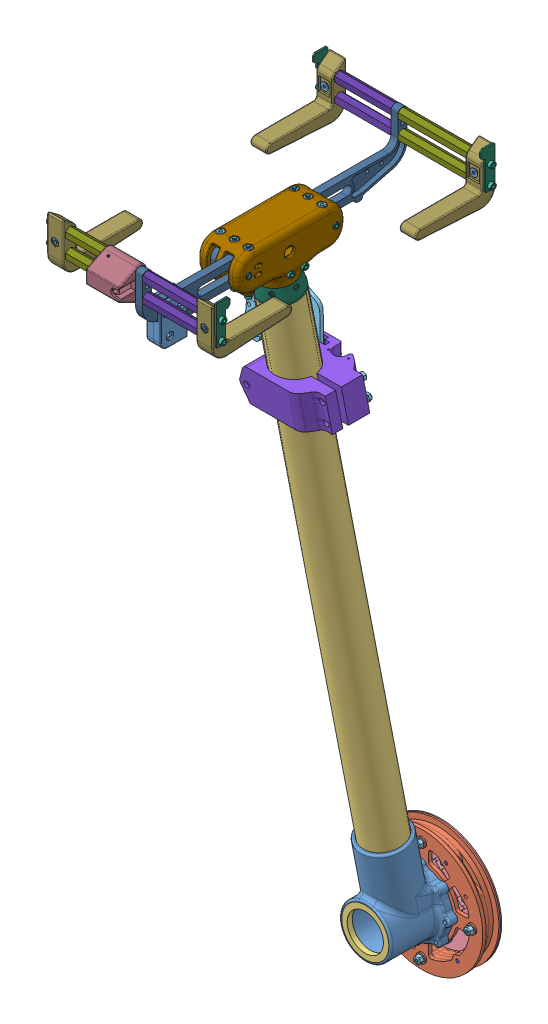
SolidWorks assembly 971-18-A-4600_Distal Arm Tubes, configuration Default. Lengths in mm.
Overall size (268.43 1098.92 452.33).
183 component instances, 51 part files, 58 mates.
Components (placement in the parent):
- 971-18-P-0131_Distal Joint End Sleeve Block-1: 971-18-P-0131_Distal Joint End Sleeve Block [Default] at origin size (98.43 160.77 84.48)
- 971-18-P-0117_Distal Joint Capstan Top -1: 971-18-P-0117_Distal Joint Capstan Top  [Distal Joint Capstan Top] at (47.625 -11.95 -3.3338) x (0 0 1) z (-0.707107 0.707107 0) size (24.51 167.64 167.64)
- 50mm x 65mm x 7mm-1: 50mm x 65mm x 7mm [Default] at (47.625 -11.95 5.3975) x (0 0 1) z (-0.033242 -0.999447 0) size (7 65 65)
- 971-18-A-2800_Capstan Tensioner-1: 971-18-A-2800_Capstan Tensioner [Default] at (81.152 21.577 -3.3338) x (0.707107 -0.707107 0) z (0 0 -1) size (57.15 30.16 17.27)
  - 971-18-P-0066_Capstan Tensioner Block-1: 971-18-P-0066_Capstan Tensioner Block [Default] at origin size (57.15 9.53 17.27)
  - Nylon-Insert Locknut-1: Nylon-Insert Locknut [#10-32  Nylon-Insert Locknut] at (-20.6375 2.032 0) x (-0.5 0 -0.866025) z (-0.866025 0 0.5) size (9.53 5.95 11)
  - SHCS-2: SHCS [0.875, #10-32] at (-20.6375 -1.5875 0) x (0 -1 0) z (-0.804306 0 -0.594216) size (27.05 7.92 7.92)
  - Nylon-Insert Locknut-2: Nylon-Insert Locknut [#10-32  Nylon-Insert Locknut] at (20.6375 2.032 0) x (0.5 0 -0.866025) z (-0.866025 0 -0.5) size (9.53 5.95 11)
  - SHCS-3: SHCS [0.875, #10-32] at (20.6375 -1.5875 0) x (0 -1 0) z (-0.804306 0 0.594216) size (27.05 7.92 7.92)
  - 3-16 in wire rope stop-1: 3-16 in wire rope stop [Default] at (5.4991 13.4938 0) x (0.991815 0 0.127683) z (-0.127683 0 0.991815) size (10.72 7.94 10.72)
  - 3-16 in wire rope stop-2: 3-16 in wire rope stop [Default] at (-5.4991 13.4938 0) x (0.997136 0 0.075631) z (-0.075631 0 0.997136) size (10.72 7.94 10.72)
- 50mm x 65mm x 7mm-2: 50mm x 65mm x 7mm [Default] at (47.625 -11.95 81.4369) x (0 0 1) z (-0.807978 0.589212 0) size (7 65 65)
- Dowel Pins-1: Dowel Pins [0.1875" OD, 0.5" Length] at (17.3166 -42.2584 11.7475) x (0 0 1) z (0.811004 0.585041 0) size (12.7 4.76 4.76)
- SHCS-1: SHCS [0.375, #10-32] at (4.7625 -11.95 10.16) x (0 0 1) z (0.375926 0.92665 0) size (14.35 7.92 7.92)
- Dowel Pins-8: Dowel Pins [0.1875" OD, 0.5" Length] at (77.9334 -42.2584 11.7475) x (0 0 1) z (-0.585041 0.811004 0) size (12.7 4.76 4.76)
- Dowel Pins-9: Dowel Pins [0.1875" OD, 0.5" Length] at (77.9334 18.3584 11.7475) x (0 0 1) z (-0.811004 -0.585041 0) size (12.7 4.76 4.76)
- Dowel Pins-10: Dowel Pins [0.1875" OD, 0.5" Length] at (17.3166 18.3584 11.7475) x (0 0 1) z (0.585041 -0.811004 0) size (12.7 4.76 4.76)
- SHCS-8: SHCS [0.375, #10-32] at (47.625 -54.8125 10.16) x (0 0 1) z (-0.92665 0.375926 0) size (14.35 7.92 7.92)
- SHCS-9: SHCS [0.375, #10-32] at (90.4875 -11.95 10.16) x (0 0 1) z (-0.375926 -0.92665 0) size (14.35 7.92 7.92)
- SHCS-10: SHCS [0.375, #10-32] at (47.625 30.9125 10.16) x (0 0 1) z (0.92665 -0.375926 0) size (14.35 7.92 7.92)
- 971-18-A-4000_The Claw-1: 971-18-A-4000_The Claw [Default] at (47.625 881.6358 218.1087) x (-1 0 0) z (0 -0.000724 1) size (243.27 530.53 410.02)
  - 971-18-P-0108_Printed Claw Body-1: 971-18-P-0108_Printed Claw Body [Default] at origin size (58.05 92.05 149.22)
  - 971-18-P-0077_Main Claw plate-2: 971-18-P-0077_Main Claw plate [Main Claw plate revised] at (9.4298 -158.75 -26.9875) x (0 0 1) z (-1 0 0) size (261.94 82.88 9.53)
  - 971-18-P-0077_Main Claw plate-3: 971-18-P-0077_Main Claw plate [Main Claw plate revised] at (-9.4298 -158.75 26.9875) x (0 0 -1) z (1 0 0) size (261.94 82.88 9.53)
  - SHCS-1: SHCS [2.25, #10-32] at (3.175 0 -60.325) x (1 0 0) z (0 0.140282 0.990112) size (61.98 7.92 7.92)
  - SHCS-2: SHCS [2.25, #10-32] at (3.175 0 60.325) x (1 0 0) z (0 0.980553 -0.196257) size (61.98 7.92 7.92)
  - SHCS-3: SHCS [1.875, #10-32] at (-19.177 -1.5875 -50.8) x (0 -1 0) z (-0.074372 0 -0.997231) size (52.45 7.92 7.92)
  - SHCS-8: SHCS [2.25, #10-32] at (0 1.5875 -50.8) x (0 -1 0) z (-0.997477 0 -0.07099) size (61.98 7.92 7.92)
  - SHCS-9: SHCS [2.25, #10-32] at (19.177 1.5875 -50.8) x (0 -1 0) z (-0.818231 0 -0.57489) size (61.98 7.92 7.92)
  - SHCS-10: SHCS [1.875, #10-32] at (19.177 -1.5875 50.8) x (0 -1 0) z (-0.72422 0 -0.689569) size (52.45 7.92 7.92)
  - SHCS-11: SHCS [2.25, #10-32] at (0 1.5875 50.8) x (0 -1 0) z (-0.999175 0 0.040609) size (61.98 7.92 7.92)
  - SHCS-12: SHCS [2.25, #10-32] at (-19.177 1.5875 50.8) x (0 -1 0) z (0.998979 0 0.045167) size (61.98 7.92 7.92)
  - 9433K640_PRECISION STAINLESS STEEL EXTENSION SPRING-1: 9433K640_PRECISION STAINLESS STEEL EXTENSION SPRING [9433K64] at (18.9548 0 -18.9695) x (0 0 1) z (-1 0 0) size (39.67 9.89 9.66)
  - 91259A155_ALLOY STEEL SHOULDER SCREW-1: 91259A155_ALLOY STEEL SHOULDER SCREW [91259A155] at (20.5423 0 -7.9375) x (0 -0.354679 -0.934988) z (0 -0.934988 0.354679) size (6.35 13.86 6.35)
  - 91259A155_ALLOY STEEL SHOULDER SCREW-2: 91259A155_ALLOY STEEL SHOULDER SCREW [91259A155] at (-20.5423 0 -34.9538) x (0 -0.751431 0.659812) z (0 -0.659812 -0.751431) size (6.35 13.86 6.35)
  - 9433K640_PRECISION STAINLESS STEEL EXTENSION SPRING-2: 9433K640_PRECISION STAINLESS STEEL EXTENSION SPRING [9433K64] at (-18.9548 0 20.6375) x (0 0 1) z (-1 0 0) size (39.67 9.89 9.66)
  - Bearings-1: Bearings [0.1875 ID, 0.375 OD, 0.125 Width, R166-2Z] at (9.3662 27.94 -18.3873) x (0 -0.996654 0.08174) z (1 0 0) size (9.53 9.53 3.17)
  - Bearings-2: Bearings [0.1875 ID, 0.375 OD, 0.125 Width, R166-2Z] at (-9.4932 27.94 1.0215) x (0 -0.380852 0.924636) z (1 0 0) size (9.53 9.53 3.17)
  - 971-18-P-0120_Printed Claw Pulley-3: 971-18-P-0120_Printed Claw Pulley [Default] at (-9.4298 27.94 1.0215) x (0 0.87562 0.483001) z (-1 0 0) size (19.05 19.05 4.76)
  - 971-18-P-0120_Printed Claw Pulley-4: 971-18-P-0120_Printed Claw Pulley [Default] at (9.4298 27.94 -18.3873) x (0 -0.06152 0.998106) z (-1 0 0) size (19.05 19.05 4.76)
  - SHCS-13: SHCS [2.25, #10-32] at (3.175 27.94 -18.3873) x (1 0 0) z (0 0.140282 0.990112) size (61.98 7.92 7.92)
  - SHCS-14: SHCS [2.25, #10-32] at (3.175 27.94 1.0215) x (1 0 0) z (0 0.140282 0.990112) size (61.98 7.92 7.92)
  - Nylon-Insert Locknut-1: Nylon-Insert Locknut [#10-32 Thin Nylon-Insert Locknut] at (22.225 27.94 1.0215) x (0 -0.5 -0.866025) z (0 -0.866025 0.5) size (9.53 4.37 11)
  - Nylon-Insert Locknut-2: Nylon-Insert Locknut [#10-32 Thin Nylon-Insert Locknut] at (22.225 27.94 -18.3873) x (0 1 0) z (0 0 -1) size (9.53 4.37 11)
  - Nylon-Insert Locknut-4: Nylon-Insert Locknut [#10-32 Thin Nylon-Insert Locknut] at (24.2094 0 -60.325) x (0 -0.5 -0.866025) z (0 -0.866025 0.5) size (9.53 4.37 11)
  - Nylon-Insert Locknut-5: Nylon-Insert Locknut [#10-32 Thin Nylon-Insert Locknut] at (24.2094 0 60.325) x (0 -0.5 0.866025) z (0 0.866025 0.5) size (9.53 4.37 11)
  - Nylon-Insert Locknut-14: Nylon-Insert Locknut [#10-32 Thin Nylon-Insert Locknut] at (19.177 -21.0344 50.8) x (0.5 0 0.866025) z (0.866025 0 -0.5) size (9.53 4.37 11)
  - Nylon-Insert Locknut-15: Nylon-Insert Locknut [#10-32 Thin Nylon-Insert Locknut] at (0 -21.0344 50.8) x (-0.5 0 -0.866025) z (-0.866025 0 0.5) size (9.53 4.37 11)
  - Nylon-Insert Locknut-17: Nylon-Insert Locknut [#10-32 Thin Nylon-Insert Locknut] at (-19.177 -21.0344 50.8) x (-0.5 0 -0.866025) z (-0.866025 0 0.5) size (9.53 4.37 11)
  - Nylon-Insert Locknut-18: Nylon-Insert Locknut [#10-32 Thin Nylon-Insert Locknut] at (0 -21.0344 -50.8) x (1 0 0) z (0 0 -1) size (9.53 4.37 11)
  - Nylon-Insert Locknut-19: Nylon-Insert Locknut [#10-32 Thin Nylon-Insert Locknut] at (-19.177 -21.0344 -50.8) x (0.5 0 -0.866025) z (-0.866025 0 -0.5) size (9.53 4.37 11)
  - Nylon-Insert Locknut-20: Nylon-Insert Locknut [#10-32 Thin Nylon-Insert Locknut] at (19.177 -21.0344 -50.8) x (-0.5 0 0.866025) z (0.866025 0 0.5) size (9.53 4.37 11)
  - 971-18-P-0142_Distal Carbon tube adapter-1: 971-18-P-0142_Distal Carbon tube adapter [Default] at (0 89.7497 -17.5007) x (-0.5 -0.165748 -0.850016) z (0 0.981514 -0.19139) size (53.98 53.98 46.99)
  - 6498K084_ROUND BODY AIR CYLINDER-1: 6498K084_ROUND BODY AIR CYLINDER [6498K084] at (0 262.1497 -57.0582) x (0 0.981514 -0.19139) z (0 0.19139 0.981514) size (365.16 28.45 28.45)
  - 5779K652_PUSH-TO-CONNECT TUBE FITTING FOR AIR-1: 5779K652_PUSH-TO-CONNECT TUBE FITTING FOR AIR [5779K652] at (0 225.7462 -44.6778) x (-1 0 0) z (0 -0.19139 -0.981514) size (14.22 28.59 25.52)
  - 971-18-P-0153_Claw Piston Mount-1: 971-18-P-0153_Claw Piston Mount [Default] at (0 207.2186 -46.3469) x (-1 0 0) z (0 -0.19139 -0.981514) size (45.75 3.17 41.53)
  - FHCS-15: FHCS [0.25, #4-40] at (-15.7499 209.7238 -50.0883) x (-0.913608 0.077818 0.39908) z (0 0.981514 -0.19139) size (6.48 6.48 6.43)
  - FHCS-18: FHCS [0.25, #4-40] at (15.7499 209.7238 -50.0883) x (-0.453098 0.170616 0.874981) z (0 0.981514 -0.19139) size (6.48 6.48 6.43)
  - FHCS-17: FHCS [0.25, #4-40] at (0 214.9449 -23.313) x (-0.453098 0.170616 0.874981) z (0 0.981514 -0.19139) size (6.48 6.48 6.43)
  - 971-18-P-0162_Claw Piston Cable Block-1: 971-18-P-0162_Claw Piston Cable Block [Default] at (0 80.0327 -21.5464) x (0.973108 0.044086 0.22609) z (-0.230348 0.186243 0.95512) size (12.7 31.75 12.7)
  - SHCS-19: SHCS [0.875, #10-32] at (0.7167 71.3508 -22.9383) x (0.230348 -0.186243 -0.95512) z (0.455328 -0.84681 0.274935) size (27.05 7.92 7.92)
  - Nylon-Insert Locknut-21: Nylon-Insert Locknut [#10-32 Thin Nylon-Insert Locknut] at (1.843 70.4402 -27.6084) x (-0.550845 -0.834076 0.029792) z (0.802191 -0.51926 0.294719) size (9.53 4.37 11)
  - SAE Washer, 18-8 Stainless Steel-1: SAE Washer, 18-8 Stainless Steel [No. 10 Screw SAE Washer] at (-1.6529 73.2667 -13.113) x (0.166548 0.974577 -0.14987) z (0.95875 -0.124551 0.25551) size (12.7 1.65 12.7)
  - SAE Washer, 18-8 Stainless Steel-2: SAE Washer, 18-8 Stainless Steel [No. 10 Screw SAE Washer] at (1.6529 70.5939 -26.8199) x (0.166548 0.974577 -0.14987) z (0.95875 -0.124551 0.25551) size (12.7 1.65 12.7)
  - FHCS-19: FHCS [0.25, #4-40] at (0 214.9449 -23.313) x (-0.309292 0.182005 0.933388) z (0 0.981514 -0.19139) size (6.48 6.48 6.43)
  - Beam Diffuse Sensor-1: Beam Diffuse Sensor [Default] at (2.3678 -35.946 191.135) x (0 -1 0) z (0 0 1) size (12.7 33.5 22.88)
  - SHCS-24: SHCS [1, #10-32] at (-103.6637 -29.5056 185.7375) x (1 0 0) z (0 0.235318 -0.971918) size (30.45 7.92 7.92)
  - SHCS-26: SHCS [1.5, #4-40] at (30.5617 -43.439 194.183) x (0 -1 0) z (0.977714 0 0.209939) size (40.94 4.65 4.65)
  - SHCS-33: SHCS [1, #10-32] at (103.6637 -29.5056 185.7375) x (-1 0 0) z (0 0.845438 -0.534073) size (30.45 7.92 7.92)
  - SHCS-35: SHCS [1, #10-32] at (103.6637 -54.9056 185.7375) x (-1 0 0) z (0 -0.631694 -0.775218) size (30.45 7.92 7.92)
  - SHCS-37: SHCS [1, #10-32] at (103.6637 -29.5056 -185.7375) x (-1 0 0) z (0 -0.058563 -0.998284) size (30.45 7.92 7.92)
  - SHCS-39: SHCS [1, #10-32] at (103.6637 -54.9056 -185.7375) x (-1 0 0) z (0 -0.744643 -0.667463) size (30.45 7.92 7.92)
  - SHCS-41: SHCS [1, #10-32] at (-103.6637 -54.9056 -185.7375) x (1 0 0) z (0 0.359883 -0.932997) size (30.45 7.92 7.92)
  - SHCS-43: SHCS [1, #10-32] at (-103.6637 -29.5056 -185.7375) x (1 0 0) z (0 0.980192 0.198051) size (30.45 7.92 7.92)
  - 92311A433_18-8 SS CUP POINT SET SCREW-1: 92311A433_18-8 SS CUP POINT SET SCREW [92311A433] at (-10.0105 -54.9056 185.7375) x (0 -0.712759 -0.701409) z (-1 0 0) size (4.99 4.84 25.82)
  - 92311A433_18-8 SS CUP POINT SET SCREW-5: 92311A433_18-8 SS CUP POINT SET SCREW [92311A433] at (-11.02 -29.5056 185.7375) x (0 -0.999929 0.011906) z (1 0 0) size (4.99 4.84 25.82)
  - 93365A142_BRASS HEAT-SET INSERT FOR PLASTICS-1: 93365A142_BRASS HEAT-SET INSERT FOR PLASTICS [93365A142] at (-11.1125 53.5447 9.169) x (0.785545 0.5 0.36458) z (0.36458 -0.850016 0.380203) size (6.35 8.46 6.35)
  - 93365A142_BRASS HEAT-SET INSERT FOR PLASTICS-2: 93365A142_BRASS HEAT-SET INSERT FOR PLASTICS [93365A142] at (-22.225 49.8609 -9.7226) x (0 0.545272 0.838259) z (0 -0.838259 0.545272) size (6.35 8.46 6.35)
  - 93365A142_BRASS HEAT-SET INSERT FOR PLASTICS-4: 93365A142_BRASS HEAT-SET INSERT FOR PLASTICS [93365A142] at (-11.1125 46.1772 -28.6142) x (-0.813186 -0.24774 0.526644) z (0.297873 -0.954543 0.010914) size (6.35 8.46 6.35)
  - 93365A142_BRASS HEAT-SET INSERT FOR PLASTICS-6: 93365A142_BRASS HEAT-SET INSERT FOR PLASTICS [93365A142] at (11.1125 46.1772 -28.6142) x (0.371763 0.927557 0.037811) z (-0.782172 0.33491 -0.525398) size (6.35 8.46 6.35)
  - 93365A142_BRASS HEAT-SET INSERT FOR PLASTICS-8: 93365A142_BRASS HEAT-SET INSERT FOR PLASTICS [93365A142] at (22.225 49.8609 -9.7226) x (0 0.873561 -0.486714) z (0 -0.486714 -0.873561) size (6.35 8.46 6.35)
  - 93365A142_BRASS HEAT-SET INSERT FOR PLASTICS-10: 93365A142_BRASS HEAT-SET INSERT FOR PLASTICS [93365A142] at (11.1125 53.5447 9.169) x (0.459987 0.780789 -0.422825) z (0.733766 -0.602409 -0.314152) size (6.35 8.46 6.35)
  - 92311A433_18-8 SS CUP POINT SET SCREW-11: 92311A433_18-8 SS CUP POINT SET SCREW [92311A433] at (9.2914 -29.5056 -185.7375) x (0 0.990314 -0.138846) z (1 0 0) size (4.99 4.84 25.82)
  - 92311A433_18-8 SS CUP POINT SET SCREW-14: 92311A433_18-8 SS CUP POINT SET SCREW [92311A433] at (9.9158 -54.9056 -185.7375) x (0 -0.994426 -0.105437) z (1 0 0) size (4.99 4.84 25.82)
  - 94638A222_NYLON UNTHREADED SPACERS-1: 94638A222_NYLON UNTHREADED SPACERS [94638A222] at (-19.177 0 50.8) x (1 0 0) z (0 1 0) size (9.53 9.53 33.34)
  - 94638A222_NYLON UNTHREADED SPACERS-2: 94638A222_NYLON UNTHREADED SPACERS [94638A222] at (-19.177 0 -50.8) x (1 0 0) z (0 1 0) size (9.53 9.53 33.34)
  - 94638A222_NYLON UNTHREADED SPACERS-3: 94638A222_NYLON UNTHREADED SPACERS [94638A222] at (19.177 0 -50.8) x (1 0 0) z (0 1 0) size (9.53 9.53 33.34)
  - 94639A550_NYLON UNTHREADED SPACERS-1: 94639A550_NYLON UNTHREADED SPACERS [94639A550] at (-9.4298 0 -60.325) x (0 -0.918334 -0.395806) z (1 0 0) size (12.7 12.7 9.53)
  - 94639A586_NYLON UNTHREADED SPACERS-1: 94639A586_NYLON UNTHREADED SPACERS [94639A586] at (0 11.9062 50.8) x (1 0 0) z (0 1 0) size (9.53 9.53 10.32)
  - 94638A222_NYLON UNTHREADED SPACERS-4: 94638A222_NYLON UNTHREADED SPACERS [94638A222] at (19.177 0 50.8) x (1 0 0) z (0 1 0) size (9.53 9.53 33.34)
  - 94639A550_NYLON UNTHREADED SPACERS-2: 94639A550_NYLON UNTHREADED SPACERS [94639A550] at (9.4298 0 -60.325) x (0 -0.323653 0.946176) z (-1 0 0) size (12.7 12.7 9.53)
  - 94639A550_NYLON UNTHREADED SPACERS-3: 94639A550_NYLON UNTHREADED SPACERS [94639A550] at (-9.4298 0 60.325) x (0 -0.362888 0.931833) z (-1 0 0) size (12.7 12.7 9.53)
  - 94639A550_NYLON UNTHREADED SPACERS-4: 94639A550_NYLON UNTHREADED SPACERS [94639A550] at (9.4298 0 60.325) x (0 -0.966697 0.255924) z (-1 0 0) size (12.7 12.7 9.53)
  - 94639A586_NYLON UNTHREADED SPACERS-2: 94639A586_NYLON UNTHREADED SPACERS [94639A586] at (0 11.9062 -50.8) x (1 0 0) z (0 1 0) size (9.53 9.53 10.32)
  - 94639A586_NYLON UNTHREADED SPACERS-3: 94639A586_NYLON UNTHREADED SPACERS [94639A586] at (0 -11.9062 50.8) x (1 0 0) z (0 1 0) size (9.53 9.53 10.32)
  - 94639A586_NYLON UNTHREADED SPACERS-4: 94639A586_NYLON UNTHREADED SPACERS [94639A586] at (0 -11.9062 -50.8) x (1 0 0) z (0 1 0) size (9.53 9.53 10.32)
  - 91780A049_ALUM FEM THRDED HEX STANDOFF-1: 91780A049_ALUM FEM THRDED HEX STANDOFF [91780A049] at (0 174.4329 -15.4133) x (0.203683 0.187378 0.960938) z (0 -0.981514 0.19139) size (6.35 7.33 76.64)
  - 98637A123_ALLOY STEEL MIL SPEC CUP POINT SET SCREW-1: 98637A123_ALLOY STEEL MIL SPEC CUP POINT SET SCREW [98637A123] at (0 134.5273 -7.632) x (0.994254 0.020488 0.105072) z (0 -0.981514 0.19139) size (3.28 2.93 13.1)
  - SHCS-44: SHCS [1, #10-32] at (-103.6637 -54.9056 185.7375) x (1 0 0) z (0 0.985655 0.168775) size (30.45 7.92 7.92)
  - 91780A049_ALUM FEM THRDED HEX STANDOFF-2: 91780A049_ALUM FEM THRDED HEX STANDOFF [91780A049] at (15.7499 94.4205 -27.6048) x (-0.911227 0.078834 0.404291) z (0 0.981514 -0.19139) size (6.35 7.33 76.64)
  - 91780A049_ALUM FEM THRDED HEX STANDOFF-3: 91780A049_ALUM FEM THRDED HEX STANDOFF [91780A049] at (-15.7499 169.2118 -42.1887) x (1 0 0) z (0 0.981514 -0.19139) size (6.35 7.33 76.64)
  - 91780A049_ALUM FEM THRDED HEX STANDOFF-4: 91780A049_ALUM FEM THRDED HEX STANDOFF [91780A049] at (-15.7499 94.4205 -27.6048) x (-0.005423 -0.191387 -0.9815) z (0 -0.981514 0.19139) size (6.35 7.33 76.64)
  - 91780A049_ALUM FEM THRDED HEX STANDOFF-5: 91780A049_ALUM FEM THRDED HEX STANDOFF [91780A049] at (15.7499 169.2118 -42.1887) x (-0.577436 0.156258 0.801344) z (0 0.981514 -0.19139) size (6.35 7.33 76.64)
  - 91780A049_ALUM FEM THRDED HEX STANDOFF-6: 91780A049_ALUM FEM THRDED HEX STANDOFF [91780A049] at (0 99.6415 -0.8294) x (0.866025 -0.095695 -0.490757) z (0 -0.981514 0.19139) size (6.35 7.33 76.64)
  - 98637A123_ALLOY STEEL MIL SPEC CUP POINT SET SCREW-2: 98637A123_ALLOY STEEL MIL SPEC CUP POINT SET SCREW [98637A123] at (-15.7499 132.8293 -35.0943) x (-0.962053 0.052223 0.267819) z (0 0.981514 -0.19139) size (3.28 2.93 13.1)
  - 98637A123_ALLOY STEEL MIL SPEC CUP POINT SET SCREW-3: 98637A123_ALLOY STEEL MIL SPEC CUP POINT SET SCREW [98637A123] at (15.7499 131.8727 -34.9077) x (-0.341225 -0.179903 -0.922605) z (0 -0.981514 0.19139) size (3.28 2.93 13.1)
  - 971-18-P-0299_Printed Claw Ends-1: 971-18-P-0299_Printed Claw Ends [Default] at (102.9652 -29.5056 -185.7375) size (22.23 68.03 110.13)
  - 971-18-P-0299_Printed Claw Ends-2: 971-18-P-0299_Printed Claw Ends [Default] at (-102.9652 -29.5056 -185.7375) size (22.23 68.03 110.13)
  - 971-18-P-0299_Printed Claw Ends-3: 971-18-P-0299_Printed Claw Ends [Default] at (-102.9652 -29.5056 185.7375) x (-1 0 0) z (0 0 -1) size (22.23 68.03 110.13)
  - 971-18-P-0299_Printed Claw Ends-4: 971-18-P-0299_Printed Claw Ends [Default] at (102.9652 -29.5056 185.7375) x (-1 0 0) z (0 0 -1) size (22.23 68.03 110.13)
  - 971-18-P-0300_Printed Claw Beam Break Mount-1: 971-18-P-0300_Printed Claw Beam Break Mount [Default] at (18.1928 -29.469 185.801) x (-1 0 0) z (0 0 -1) size (45.72 44.45 38.48)
  - Nylon-Insert Locknut-22: Nylon-Insert Locknut [#10-32 Thin Nylon-Insert Locknut] at (102.9652 -42.2056 190.5) x (-0.998457 -0.055527 0) z (-0.055527 0.998457 0) size (9.53 4.37 11)
  - FHCS-20: FHCS [0.75, #10-32] at (102.9652 -42.2056 176.2125) x (-0.923728 -0.383049 0) z (0 0 -1) size (10.44 10.44 19.21)
  - FHCS-21: FHCS [0.75, #10-32] at (-102.9652 -42.2056 176.2125) x (-0.873774 -0.486332 0) z (0 0 -1) size (10.44 10.44 19.21)
  - FHCS-24: FHCS [0.75, #10-32] at (-102.9652 -42.2056 -176.2125) x (-0.044015 -0.999031 0) z (0 0 1) size (10.44 10.44 19.21)
  - FHCS-26: FHCS [0.75, #10-32] at (102.9652 -42.2056 -176.2125) x (0.130134 -0.991496 0) z (0 0 1) size (10.44 10.44 19.21)
  - Nylon-Insert Locknut-23: Nylon-Insert Locknut [#10-32 Thin Nylon-Insert Locknut] at (-102.9652 -42.2056 190.5) x (-0.985526 -0.169524 0) z (-0.169524 0.985526 0) size (9.53 4.37 11)
  - Nylon-Insert Locknut-25: Nylon-Insert Locknut [#10-32 Thin Nylon-Insert Locknut] at (-102.9652 -42.2056 -190.5) x (0.289314 -0.957234 0) z (0.957234 0.289314 0) size (9.53 4.37 11)
  - Nylon-Insert Locknut-27: Nylon-Insert Locknut [#10-32 Thin Nylon-Insert Locknut] at (102.9652 -42.2056 -190.5) x (0.451141 -0.892453 0) z (0.892453 0.451141 0) size (9.53 4.37 11)
  - 971-18-P-0304_Claw Standoff Ring-1: 971-18-P-0304_Claw Standoff Ring [Default] at (0 65.555 -12.7829) x (0.5 0.165748 0.850016) z (-0.866025 0.095695 0.490757) size (43.02 19.34 44.45)
  - 971-18-P-0312_Claw Fangs-1: 971-18-P-0312_Claw Fangs [Default] at (114.0778 -76.4956 200.7755) size (2.29 53.34 19.05) (hidden)
  - 971-18-P-0312_Claw Fangs-6: 971-18-P-0312_Claw Fangs [Default] at (-114.0778 -76.4956 -200.7755) x (-1 0 0) z (0 0 -1) size (2.29 53.34 19.05)
  - 971-18-P-0312_Claw Fangs-11: 971-18-P-0312_Claw Fangs [Default] at (116.3637 -76.4956 -200.7755) x (-1 0 0) z (0 0 -1) size (2.29 53.34 19.05)
  - 971-18-P-0312_Claw Fangs-12: 971-18-P-0312_Claw Fangs [Default] at (-116.3637 -76.4956 200.7755) size (2.29 53.34 19.05)
  - 971-18-P-0316_Claw Long Horizontal Standoff-1: 971-18-P-0316_Claw Long Horizontal Standoff [91780A354] at (-46.1328 -54.9056 -185.7375) x (0 0.866025 -0.5) z (1 0 0) size (12.7 14.66 102.22)
  - 971-18-P-0317_Claw Short Horizontal Standoff-1: 971-18-P-0317_Claw Short Horizontal Standoff [91780A354] at (-91.8528 -54.9056 185.7375) x (0 -0.912023 0.41014) z (1 0 0) size (12.7 14.66 82.74)
  - 971-18-P-0317_Claw Short Horizontal Standoff-2: 971-18-P-0317_Claw Short Horizontal Standoff [91780A354] at (91.8528 -54.9056 -185.7375) x (0 -0.866025 0.5) z (-1 0 0) size (12.7 14.66 82.74)
  - 971-18-P-0317_Claw Short Horizontal Standoff-3: 971-18-P-0317_Claw Short Horizontal Standoff [91780A354] at (91.8528 -29.5056 -185.7375) x (0 0.196892 -0.980425) z (-1 0 0) size (12.7 14.66 82.74)
  - 971-18-P-0317_Claw Short Horizontal Standoff-4: 971-18-P-0317_Claw Short Horizontal Standoff [91780A354] at (-91.8528 -29.5056 185.7375) x (0 0.866025 -0.5) z (1 0 0) size (12.7 14.66 82.74)
  - 971-18-P-0316_Claw Long Horizontal Standoff-2: 971-18-P-0316_Claw Long Horizontal Standoff [91780A354] at (46.1328 -29.5056 185.7375) x (0 0 1) z (-1 0 0) size (12.7 14.66 102.22)
  - 971-18-P-0316_Claw Long Horizontal Standoff-3: 971-18-P-0316_Claw Long Horizontal Standoff [91780A354] at (-46.1328 -29.5056 -185.7375) x (0 0.866025 -0.5) z (1 0 0) size (12.7 14.66 102.22)
  - 971-18-P-0316_Claw Long Horizontal Standoff-4: 971-18-P-0316_Claw Long Horizontal Standoff [91780A354] at (46.1328 -54.9056 185.7375) x (0 0.866025 -0.5) z (-1 0 0) size (12.7 14.66 102.22)
  - 971-18-P-0326_Claw Cable Holder-2: 971-18-P-0326_Claw Cable Holder [Default] at (-19.177 30.1625 50.8) x (1 0 0) z (0 0 -1) size (30.61 4.76 11.43)
  - 971-18-P-0326_Claw Cable Holder-3: 971-18-P-0326_Claw Cable Holder [Default] at (0 30.1625 -50.8) x (1 0 0) z (0 0 -1) size (30.61 4.76 11.43)
  - 971-18-P-0318_Claw Pulley Mount-5: 971-18-P-0318_Claw Pulley Mount [971-18-P-0318_Claw Pulley Mount] at (-19.2722 5.212 171.7608) x (0 0 -1) z (1 0 0) size (36.91 55.31 10.39)
  - 971-18-P-0318_Claw Pulley Mount-6: 971-18-P-0318_Claw Pulley Mount [971-18-P-0330_Claw Pulley Mount Inner Side] at (-9.4298 5.212 171.7608) x (0 0 -1) z (1 0 0) size (36.91 55.31 11.43)
  - 971-18-P-0361_Claw Fangs V2-1: 971-18-P-0361_Claw Fangs V2 [Default] at (115.2207 -29.5056 185.7375) size (2.29 63.5 20.32)
  - 971-18-P-0367_Retrofit Fang Sheath-1: 971-18-P-0367_Retrofit Fang Sheath [Default] at (116.3637 -29.5056 185.7375) x (1 0 0) z (0 -0.027695 0.999616) size (1.52 70.53 41.08)
  - 971-18-P-0368_Retrofit Fang Sheath Outside-1: 971-18-P-0368_Retrofit Fang Sheath Outside [Default] at (120.3325 -29.5056 185.7375) size (1.52 74.51 17.53)
- Dowel Pins-11: Dowel Pins [0.1875" OD, 1" Length] at (-1.3174 36.9924 -2.54) x (0 0 1) z (-0.585041 0.811004 0) size (25.4 4.76 4.76)
- Dowel Pins-12: Dowel Pins [0.1875" OD, 1" Length] at (80.8519 48.2177 -2.54) x (0 0 1) z (-0.585041 0.811004 0) size (25.4 4.76 4.76)
- Dowel Pins-13: Dowel Pins [0.1875" OD, 1" Length] at (-1.3174 -60.8924 -2.54) x (0 0 1) z (-0.585041 0.811004 0) size (25.4 4.76 4.76)
- Dowel Pins-14: Dowel Pins [0.1875" OD, 1" Length] at (96.5674 -60.8924 -2.54) x (0 0 1) z (-0.585041 0.811004 0) size (25.4 4.76 4.76)
- SHCS-11: SHCS [1.25, #10-32] at (-21.59 -11.95 1.524) x (0 0 1) z (-0.92665 0.375926 0) size (36.8 7.92 7.92)
- SHCS-12: SHCS [1.25, #10-32] at (47.625 -81.165 1.524) x (0 0 1) z (-0.92665 0.375926 0) size (36.8 7.92 7.92)
- SHCS-13: SHCS [1.25, #10-32] at (47.625 57.265 1.524) x (0 0 1) z (-0.92665 0.375926 0) size (36.8 7.92 7.92)
- SHCS-14: SHCS [1.25, #10-32] at (116.84 -11.95 1.524) x (0 0 1) z (-0.92665 0.375926 0) size (36.8 7.92 7.92)
- 91525A318_No8 Oversized Washer-1: 91525A318_No8 Oversized Washer [91525A318] at (47.625 57.265 10.16) x (0 0 1) z (-1 0 0) size (2.03 12.7 12.7)
- Nylon-Insert Locknut-1: Nylon-Insert Locknut [#8-32  Nylon-Insert Locknut] at (116.84 -11.95 12.192) x (1 0 0) z (0 -1 0) size (8.73 5.95 10.08)
- Nylon-Insert Locknut-4: Nylon-Insert Locknut [#8-32  Nylon-Insert Locknut] at (47.625 57.265 12.192) x (0.433349 -0.901226 0) z (-0.901226 -0.433349 0) size (8.73 5.95 10.08)
- Nylon-Insert Locknut-5: Nylon-Insert Locknut [#8-32  Nylon-Insert Locknut] at (-21.59 -11.95 12.192) x (0.56381 0.825904 0) z (0.825904 -0.56381 0) size (8.73 5.95 10.08)
- Nylon-Insert Locknut-6: Nylon-Insert Locknut [#8-32  Nylon-Insert Locknut] at (47.625 -81.165 12.192) x (0.837709 -0.546117 0) z (-0.546117 -0.837709 0) size (8.73 5.95 10.08)
- 91525A318_No8 Oversized Washer-2: 91525A318_No8 Oversized Washer [91525A318] at (116.84 -11.95 12.192) x (0 0 -1) z (-0.707107 -0.707107 0) size (2.03 12.7 12.7)
- 91525A318_No8 Oversized Washer-3: 91525A318_No8 Oversized Washer [91525A318] at (-21.59 -11.95 12.192) x (0 0 -1) z (-0.707107 -0.707107 0) size (2.03 12.7 12.7)
- 91525A318_No8 Oversized Washer-4: 91525A318_No8 Oversized Washer [91525A318] at (47.625 -81.165 12.192) x (0 0 -1) z (0.944724 0.327866 0) size (2.03 12.7 12.7)
- 971-18-P-0121_Distal Arm Carbon Fiber -1: 971-18-P-0121_Distal Arm Carbon Fiber  [Default] at (47.625 816.8258 205.4224) x (-0.927261 0.071926 -0.367443) z (0 0.981375 0.192101) size (53.98 53.98 819.15)
- 971-18-P-0308_Arm Pinch Guard 1-1: 971-18-P-0308_Arm Pinch Guard 1 [Default] at (47.625 -11.95 -15.9385) x (-1 0 0) z (0 0 1) size (167.64 167.64 1.59)
- 971-18-A-7000_Hook Deploy 2-1: 971-18-A-7000_Hook Deploy 2 [Default] at (107.95 665.743 180.8204) x (0 0 1) z (-1 0 0) size (105.09 189.79 207.33)
  - 971-18-P-0141_Hook-1: 971-18-P-0141_Hook [971-18-P-0141_Hook] at (-41.275 -386.5783 192.1852) x (1 0 0) z (0 0.620152 0.784482) size (4.76 138.46 130.88)
  - 971-18-P-0141_Hook-2: 971-18-P-0141_Hook [971-18-P-0339_Hook Deploy Bar Latch  ] at (-38.1 -387.3352 177.5272) x (1 0 0) z (0 0.591782 0.806098) size (3.18 49.73 57)
  - 971-18-P-0141_Hook-3: 971-18-P-0141_Hook [971-18-P-0339_Hook Deploy Bar Latch  ] at (-65.0875 -387.3352 177.5272) x (1 0 0) z (0 0.591782 0.806098) size (3.18 49.73 57)
  - SHCS-1: SHCS [1.5, #8-32] at (-43.0848 23.9496 163.6395) x (-1 0 0) z (0 0.313417 0.949616) size (42.27 6.86 6.86)
  - SAE Washer, 18-8 Stainless Steel-1: SAE Washer, 18-8 Stainless Steel [No. 8 Screw SAE Washer] at (-24.8603 23.9496 163.6395) x (0 0.996559 0.082881) z (0 0.082881 -0.996559) size (11.13 1.65 11.13)
  - Nylon-Insert Locknut-1: Nylon-Insert Locknut [#8-32 Thin Nylon-Insert Locknut] at (-56.8642 23.9496 163.6395) x (0 0.411961 0.911202) z (0 -0.911202 0.411961) size (8.73 4.37 10.08)
  - SHCS-2: SHCS [1.5, #8-32] at (-43.0847 37.6911 160.4371) x (-1 0 0) z (0 -0.998173 0.060419) size (42.27 6.86 6.86)
  - Nylon-Insert Locknut-2: Nylon-Insert Locknut [#8-32 Thin Nylon-Insert Locknut] at (-56.8642 37.6911 160.4371) x (0 -0.317303 -0.948324) z (0 0.948324 -0.317303) size (8.73 4.37 10.08)
  - 6604K110_MINIATURE THREADED-BODY AIR CYLINDER (1)-1: 6604K110_MINIATURE THREADED-BODY AIR CYLINDER (1) [6604K11] at (-41.275 4.8846 43.7936) x (0 1 0) z (-0.866025 0 0.5) size (46.38 18.33 15.88)
  - SHCS-5: SHCS [3.5, #8-32] at (-16.383 25.4 96.3706) x (-1 0 0) z (0 -0.99808 0.061931) size (93.07 6.86 6.86)
  - SHCS-6: SHCS [2.25, #8-32] at (-18.8323 11.1125 9.525) x (-1 0 0) z (0 0.996252 -0.086496) size (61.32 6.86 6.86)
  - SHCS-7: SHCS [2.25, #8-32] at (-11.8467 39.6875 9.525) x (-1 0 0) z (0 -0.304537 -0.9525) size (61.32 6.86 6.86)
  - 10_32-elbow-male-1_4-1: 10_32-elbow-male-1_4 [07-32] at (-41.275 -27.3504 43.7936) x (-0.221782 0 0.975096) z (0.975096 0 0.221782) size (19.44 21.55 11.1)
  - 971-18-P-0336_Hook Deploy 2 Clamp-4: 971-18-P-0336_Hook Deploy 2 Clamp [971-18-P-0338_Hook Deploy 2 Piston Cover  ] at (0 25.4 22.225) x (0 0 1) z (-1 0 0) size (105.9 50.8 99.43)
  - 6498K551_5-40 Clevis Pin-1: 6498K551_5-40 Clevis Pin [6498K551] at (-41.275 19.1086 43.7936) x (-1 0 0) z (0 0 -1) size (12.7 18.59 7.87)
  - 971-18-P-0349_Hook Deploy 2 Latch-2: 971-18-P-0349_Hook Deploy 2 Latch [Default] at (-40.132 6.35 62.0395) x (-1 0 0) z (0 0 -1) size (2.29 17.78 24.97)
  - Nylon-Insert Locknut-12: Nylon-Insert Locknut [#8-32 Thin Nylon-Insert Locknut] at (-50.3153 25.4 96.3706) x (0 -0.503678 -0.863892) z (0 0.863892 -0.503678) size (8.73 4.37 10.08)
  - Nylon-Insert Locknut-13: Nylon-Insert Locknut [#8-32 Thin Nylon-Insert Locknut] at (-35.2049 39.6875 9.525) x (0 0.782456 0.622706) z (0 -0.622706 0.782456) size (8.73 4.37 10.08)
  - Nylon-Insert Locknut-15: Nylon-Insert Locknut [#8-32 Thin Nylon-Insert Locknut] at (-42.6232 11.1125 9.525) x (0 -0.484836 0.874605) z (0 -0.874605 -0.484836) size (8.73 4.37 10.08)
  - 90145A882_18-8 STAINLESS STEEL DOWEL PIN-1: 90145A882_18-8 STAINLESS STEEL DOWEL PIN [90145A882] at (-41.6111 33.655 57.7215) x (1 0 0) z (0 -0.852468 -0.522779) size (28.57 3.17 3.17)
  - SAE Washer, 18-8 Stainless Steel-2: SAE Washer, 18-8 Stainless Steel [No. 8 Screw SAE Washer] at (-24.8603 37.6911 160.4371) x (0 0.996559 0.082881) z (0 0.082881 -0.996559) size (11.13 1.65 11.13)
  - 971-18-P-0351_Hanger Latch Pivot Spacer -1: 971-18-P-0351_Hanger Latch Pivot Spacer  [Default] at (-38.8937 37.6911 160.4371) x (0 0.144685 0.989478) z (-1 0 0) size (9.53 9.53 13.21)
  - 971-18-P-0351_Hanger Latch Pivot Spacer -2: 971-18-P-0351_Hanger Latch Pivot Spacer  [Default] at (-43.6562 37.6911 160.4371) x (0 0.973902 -0.226968) z (1 0 0) size (9.53 9.53 13.21)
  - 971-18-P-0351_Hanger Latch Pivot Spacer -3: 971-18-P-0351_Hanger Latch Pivot Spacer  [Default] at (-43.6562 23.9496 163.6395) x (0 0.973902 -0.226968) z (1 0 0) size (9.53 9.53 13.21)
  - 971-18-P-0351_Hanger Latch Pivot Spacer -4: 971-18-P-0351_Hanger Latch Pivot Spacer  [Default] at (-38.8937 23.9496 163.6395) x (0 -0.930262 0.366895) z (-1 0 0) size (9.53 9.53 13.21)
Mates (geometry in assembly coordinates):
- Coincident2: coincident anti-aligned: plane of 971-18-P-0117_Distal Joint Capstan Top -1 through (73.9229 46.7666 -14.351) normal (-0.707107 -0.707107 0); plane of 971-18-A-2800_Capstan Tensioner-1/SHCS-2 through (75.5393 45.1502 -3.3338) normal (0.707107 0.707107 0)
- Width1: width aligned: plane of 971-18-P-0117_Distal Joint Capstan Top -1 through (47.625 -11.95 5.3975) normal (0 0 -1); plane of 971-18-A-2800_Capstan Tensioner-1/971-18-P-0066_Capstan Tensioner Block-1 through (47.625 -11.95 -12.065) normal (0 0 1); plane of 971-18-P-0117_Distal Joint Capstan Top -1 through (54.2112 35.0474 -11.9698) normal (0 0 -1); plane of 971-18-A-2800_Capstan Tensioner-1/971-18-P-0066_Capstan Tensioner Block-1 through (54.2112 35.0474 5.3022) normal (0 0 1)
- Concentric10: concentric aligned: cylinder of 971-18-P-0131_Distal Joint End Sleeve Block-1 through (47.625 -11.95 88.4369) axis (0 0 -1) radius 32.5; cylinder of 50mm x 65mm x 7mm-2 through (47.625 -11.95 88.4369) axis (0 0 -1) radius 32.5
- Coincident13: coincident anti-aligned: plane of 971-18-P-0131_Distal Joint End Sleeve Block-1 through (47.625 -11.95 81.4369) normal (0 0 1); plane of 50mm x 65mm x 7mm-2 through (47.625 -11.95 81.4369) normal (0 0 -1)
- Coincident14: coordinate: point of 971-18-P-0131_Distal Joint End Sleeve Block-1; point of assembly
- Concentric11: concentric anti-aligned: cylinder of 971-18-P-0131_Distal Joint End Sleeve Block-1 through (47.625 -11.95 0) axis (0 0 1) radius 29.4925; cylinder of 50mm x 65mm x 7mm-1 through (47.625 -11.95 12.3975) axis (0 0 -1) radius 25
- Coincident15: coincident anti-aligned: plane of 971-18-P-0117_Distal Joint Capstan Top -1 through (47.625 -11.95 -3.3338) normal (-0.707107 0.707107 0); plane of 971-18-A-2800_Capstan Tensioner-1 through (81.152 21.577 -3.3338) normal (0.707107 -0.707107 0)
- Concentric16: concentric aligned: cylinder of 971-18-P-0117_Distal Joint Capstan Top -1 through (17.3166 -42.2584 -14.351) axis (0 0 1) radius 2.286; cylinder of Dowel Pins-1 through (17.3166 -42.2584 5.3975) axis (0 0 1) radius 2.3813
- Concentric18: concentric aligned: cylinder of 971-18-P-0117_Distal Joint Capstan Top -1 through (4.7625 -11.95 -14.351) axis (0 0 1) radius 2.4892; cylinder of SHCS-1 through (4.7625 -11.95 5.3975) axis (0 0 1) radius 3.9624
- Coincident21: coincident aligned: plane of 971-18-P-0117_Distal Joint Capstan Top -1 through (47.625 -11.95 5.3975) normal (0 0 -1); plane of Dowel Pins-1 through (17.3166 -42.2584 5.3975) normal (0 0 -1)
- Coincident22: coincident aligned: plane of 971-18-P-0117_Distal Joint Capstan Top -1 through (47.625 -11.95 5.3975) normal (0 0 -1); plane of 50mm x 65mm x 7mm-1 through (47.625 -11.95 5.3975) normal (0 0 -1)
- Coincident23: coincident anti-aligned: plane of 971-18-P-0117_Distal Joint Capstan Top -1 through (47.625 -11.95 5.3975) normal (0 0 -1); plane of SHCS-9 through (87.0393 -10.5511 5.3975) normal (0 0 1)
- Coincident24: coincident anti-aligned: plane of 971-18-P-0131_Distal Joint End Sleeve Block-1 through (47.625 -11.95 12.3975) normal (0 0 -1); plane of 50mm x 65mm x 7mm-1 through (47.625 -11.95 12.3975) normal (0 0 1)
- Concentric19: concentric aligned: cylinder of 971-18-P-0117_Distal Joint Capstan Top -1 through (77.9334 -42.2584 -14.351) axis (0 0 1) radius 2.286; cylinder of Dowel Pins-8 through (77.9334 -42.2584 5.3975) axis (0 0 1) radius 2.3813
- Concentric20: concentric anti-aligned: cylinder of 971-18-P-0131_Distal Joint End Sleeve Block-1 through (47.625 30.9125 133.0803) axis (0 0 -1) radius 6.35; cylinder of SHCS-10 through (47.625 30.9125 5.3975) axis (0 0 1) radius 3.9624
- Parallel1: parallel anti-aligned: plane of 971-18-A-4000_The Claw-1 through (47.625 881.6358 218.1087) normal (-1 0 0); plane of assembly through (0 0 0) normal (1 0 0)
- Concentric22: concentric anti-aligned: cylinder of 971-18-P-0117_Distal Joint Capstan Top -1 through (96.5674 -60.8924 7.6835) axis (0 0 -1) radius 2.286; cylinder of Dowel Pins-14 through (96.5674 -60.8924 -15.24) axis (0 0 1) radius 2.3813
- Coincident26: coincident aligned: plane of 971-18-P-0117_Distal Joint Capstan Top -1 through (47.625 -11.95 10.16) normal (0 0 1); plane of Dowel Pins-14 through (96.5674 -60.8924 10.16) normal (0 0 1)
- Concentric23: concentric anti-aligned: cylinder of 971-18-P-0117_Distal Joint Capstan Top -1 through (-1.3174 -60.8924 7.6835) axis (0 0 -1) radius 2.286; cylinder of Dowel Pins-13 through (-1.3174 -60.8924 -15.24) axis (0 0 1) radius 2.3813
- Coincident27: coincident aligned: plane of 971-18-P-0117_Distal Joint Capstan Top -1 through (47.625 -11.95 10.16) normal (0 0 1); plane of Dowel Pins-13 through (-1.3174 -60.8924 10.16) normal (0 0 1)
- Concentric24: concentric anti-aligned: cylinder of 971-18-P-0117_Distal Joint Capstan Top -1 through (-1.3174 36.9924 7.6835) axis (0 0 -1) radius 2.286; cylinder of Dowel Pins-11 through (-1.3174 36.9924 -15.24) axis (0 0 1) radius 2.3813
- Coincident28: coincident aligned: plane of 971-18-P-0117_Distal Joint Capstan Top -1 through (47.625 -11.95 10.16) normal (0 0 1); plane of Dowel Pins-11 through (-1.3174 36.9924 10.16) normal (0 0 1)
- Concentric25: concentric anti-aligned: cylinder of 971-18-P-0117_Distal Joint Capstan Top -1 through (80.8519 48.2177 7.6835) axis (0 0 -1) radius 2.286; cylinder of Dowel Pins-12 through (80.8519 48.2177 -15.24) axis (0 0 1) radius 2.3813
- Coincident29: coincident aligned: plane of 971-18-P-0117_Distal Joint Capstan Top -1 through (47.625 -11.95 10.16) normal (0 0 1); plane of Dowel Pins-12 through (80.8519 48.2177 10.16) normal (0 0 1)
- Coincident30: coincident anti-aligned: plane of 971-18-P-0117_Distal Joint Capstan Top -1 through (47.625 -11.95 -14.351) normal (0 0 -1); plane of SHCS-13 through (49.0239 60.7132 -14.351) normal (0 0 1)
- Coincident31: coincident anti-aligned: plane of 971-18-P-0117_Distal Joint Capstan Top -1 through (47.625 -11.95 -14.351) normal (0 0 -1); plane of SHCS-11 through (-20.1911 -8.5018 -14.351) normal (0 0 1)
- Coincident32: coincident anti-aligned: plane of 971-18-P-0117_Distal Joint Capstan Top -1 through (47.625 -11.95 -14.351) normal (0 0 -1); plane of SHCS-14 through (118.2389 -8.5018 -14.351) normal (0 0 1)
- Coincident33: coincident anti-aligned: plane of 971-18-P-0117_Distal Joint Capstan Top -1 through (47.625 -11.95 -14.351) normal (0 0 -1); plane of SHCS-12 through (49.0239 -77.7168 -14.351) normal (0 0 1)
- Concentric27: concentric aligned: cylinder of 971-18-P-0117_Distal Joint Capstan Top -1 through (116.84 -11.95 -0.9525) axis (0 0 1) radius 2.4892; cylinder of SHCS-14 through (116.84 -11.95 -14.351) axis (0 0 1) radius 2.413
- Concentric28: concentric aligned: cylinder of 971-18-P-0117_Distal Joint Capstan Top -1 through (47.625 -81.165 -0.9525) axis (0 0 1) radius 2.4892; cylinder of SHCS-12 through (47.625 -81.165 -14.351) axis (0 0 1) radius 2.413
- Concentric29: concentric aligned: cylinder of 971-18-P-0117_Distal Joint Capstan Top -1 through (47.625 57.265 -0.9525) axis (0 0 1) radius 2.4892; cylinder of SHCS-13 through (47.625 57.265 -14.351) axis (0 0 1) radius 2.413
- Concentric30: concentric aligned: cylinder of 971-18-P-0117_Distal Joint Capstan Top -1 through (-21.59 -11.95 -0.9525) axis (0 0 1) radius 2.4892; cylinder of SHCS-11 through (-21.59 -11.95 -14.351) axis (0 0 1) radius 2.413
- Coincident37: coincident anti-aligned: plane of 971-18-P-0117_Distal Joint Capstan Top -1 through (47.625 -11.95 10.16) normal (0 0 1); plane of 91525A318_No8 Oversized Washer-4 through (47.625 -81.165 10.16) normal (0 0 -1)
- Concentric34: concentric aligned: cylinder of SHCS-12 through (47.625 -81.165 -14.351) axis (0 0 1) radius 2.413; cylinder of 91525A318_No8 Oversized Washer-4 through (47.625 -81.165 10.16) axis (0 0 1) radius 2.1844
- Coincident38: coincident anti-aligned: plane of Nylon-Insert Locknut-6 through (52.6586 -81.4377 12.192) normal (0 0 -1); plane of 91525A318_No8 Oversized Washer-4 through (47.625 -81.165 12.192) normal (0 0 1)
- Concentric35: concentric anti-aligned: cylinder of SHCS-12 through (47.625 -81.165 -14.351) axis (0 0 1) radius 2.413; cylinder of Nylon-Insert Locknut-6 through (47.625 -81.165 10.1092) axis (0 0 -1) radius 2.0828
- Coincident39: coincident anti-aligned: plane of 971-18-P-0117_Distal Joint Capstan Top -1 through (47.625 -11.95 10.16) normal (0 0 1); plane of 91525A318_No8 Oversized Washer-3 through (-21.59 -11.95 10.16) normal (0 0 -1)
- Concentric36: concentric aligned: cylinder of SHCS-11 through (-21.59 -11.95 -14.351) axis (0 0 1) radius 2.413; cylinder of 91525A318_No8 Oversized Washer-3 through (-21.59 -11.95 10.16) axis (0 0 1) radius 2.1844
- Coincident40: coincident anti-aligned: plane of 971-18-P-0117_Distal Joint Capstan Top -1 through (47.625 -11.95 10.16) normal (0 0 1); plane of 91525A318_No8 Oversized Washer-2 through (116.84 -11.95 10.16) normal (0 0 -1)
- Concentric37: concentric aligned: cylinder of SHCS-14 through (116.84 -11.95 -14.351) axis (0 0 1) radius 2.413; cylinder of 91525A318_No8 Oversized Washer-2 through (116.84 -11.95 10.16) axis (0 0 1) radius 2.1844
- Coincident41: coincident anti-aligned: plane of Nylon-Insert Locknut-1 through (121.2056 -9.4295 12.192) normal (0 0 -1); plane of 91525A318_No8 Oversized Washer-2 through (116.84 -11.95 12.192) normal (0 0 1)
- Concentric38: concentric anti-aligned: cylinder of SHCS-14 through (116.84 -11.95 -14.351) axis (0 0 1) radius 2.413; cylinder of Nylon-Insert Locknut-1 through (116.84 -11.95 10.1092) axis (0 0 -1) radius 2.0828
- Coincident42: coincident anti-aligned: plane of 971-18-P-0117_Distal Joint Capstan Top -1 through (47.625 -11.95 10.16) normal (0 0 1); plane of 91525A318_No8 Oversized Washer-1 through (47.625 57.265 10.16) normal (0 0 -1)
- Concentric39: concentric anti-aligned: cylinder of SHCS-13 through (47.625 57.265 -14.351) axis (0 0 1) radius 2.413; cylinder of 91525A318_No8 Oversized Washer-1 through (47.625 57.265 12.192) axis (0 0 -1) radius 2.1844
- Coincident43: coincident anti-aligned: plane of 91525A318_No8 Oversized Washer-1 through (47.625 57.265 12.192) normal (0 0 1); plane of Nylon-Insert Locknut-4 through (51.7884 54.4228 12.192) normal (0 0 -1)
- Concentric40: concentric anti-aligned: cylinder of SHCS-13 through (47.625 57.265 -14.351) axis (0 0 1) radius 2.413; cylinder of Nylon-Insert Locknut-4 through (47.625 57.265 10.1092) axis (0 0 -1) radius 2.0828
- Coincident44: coincident anti-aligned: plane of Nylon-Insert Locknut-5 through (-21.2103 -6.9233 12.192) normal (0 0 -1); plane of 91525A318_No8 Oversized Washer-3 through (-21.59 -11.95 12.192) normal (0 0 1)
- Concentric41: concentric anti-aligned: cylinder of SHCS-11 through (-21.59 -11.95 -14.351) axis (0 0 1) radius 2.413; cylinder of Nylon-Insert Locknut-5 through (-21.59 -11.95 10.1092) axis (0 0 -1) radius 2.0828
- Concentric42: concentric aligned: cylinder of 971-18-P-0131_Distal Joint End Sleeve Block-1 through (47.625 93.9447 63.9211) axis (0 -0.981375 -0.192101) radius 26.9875; cylinder of 971-18-P-0121_Distal Arm Carbon Fiber -1 through (47.625 816.8258 205.4224) axis (0 -0.981375 -0.192101) radius 26.9875
- Coincident45: coincident anti-aligned: plane of 971-18-P-0131_Distal Joint End Sleeve Block-1 through (47.625 12.9322 48.0632) normal (0 0.981375 0.192101); plane of 971-18-P-0121_Distal Arm Carbon Fiber -1 through (38.1148 8.4078 71.1769) normal (0 -0.981375 -0.192101)
- Coincident46: coincident anti-aligned: plane of 971-18-A-4000_The Claw-1/971-18-P-0142_Distal Carbon tube adapter-1 through (70.9969 814.2336 218.6648) normal (0 -0.981375 -0.192101); plane of 971-18-P-0121_Distal Arm Carbon Fiber -1 through (38.1148 812.3013 228.5361) normal (0 0.981375 0.192101)
- Concentric43: concentric aligned: cylinder of 971-18-A-4000_The Claw-1/971-18-P-0142_Distal Carbon tube adapter-1 through (47.625 791.8988 200.543) axis (0 -0.981375 -0.192101) radius 26.9875; cylinder of 971-18-P-0121_Distal Arm Carbon Fiber -1 through (47.625 816.8258 205.4224) axis (0 -0.981375 -0.192101) radius 26.9875
- Coincident49: coincident anti-aligned: plane of 971-18-P-0117_Distal Joint Capstan Top -1 through (47.625 -11.95 -14.351) normal (0 0 -1); plane of 971-18-P-0308_Arm Pinch Guard 1-1 through (47.625 -11.95 -14.351) normal (0 0 1)
- Concentric13: concentric anti-aligned: circle of 971-18-P-0117_Distal Joint Capstan Top -1; circle of 971-18-P-0308_Arm Pinch Guard 1-1
- Concentric15: concentric aligned: circle of SHCS-12; circle of 971-18-P-0308_Arm Pinch Guard 1-1
- Concentric44: concentric aligned: cylinder of 971-18-P-0121_Distal Arm Carbon Fiber -1 through (47.625 816.8258 205.4224) axis (0 -0.981375 -0.192101) radius 26.9875; cylinder of 971-18-A-7000_Hook Deploy 2-1/971-18-P-0336_Hook Deploy 2 Clamp-4 through (47.625 691.143 180.8204) axis (0 -0.981375 -0.192101) radius 27.1145
- Parallel2: parallel aligned: plane of 971-18-A-4000_The Claw-1/971-18-P-0108_Printed Claw Body-1 through (76.2 881.6358 218.1087) normal (1 0 0); plane of 971-18-A-7000_Hook Deploy 2-1/971-18-P-0336_Hook Deploy 2 Clamp-4 through (107.95 524.2862 250.6704) normal (1 0 0)
- Distance1: distance = 190.5 mm aligned: point of 971-18-A-7000_Hook Deploy 2-1/971-18-P-0336_Hook Deploy 2 Clamp-4; plane of 971-18-A-4000_The Claw-1/971-18-P-0108_Printed Claw Body-1 through (19.05 906.9817 292.7396) normal (0 1 0.000724)
